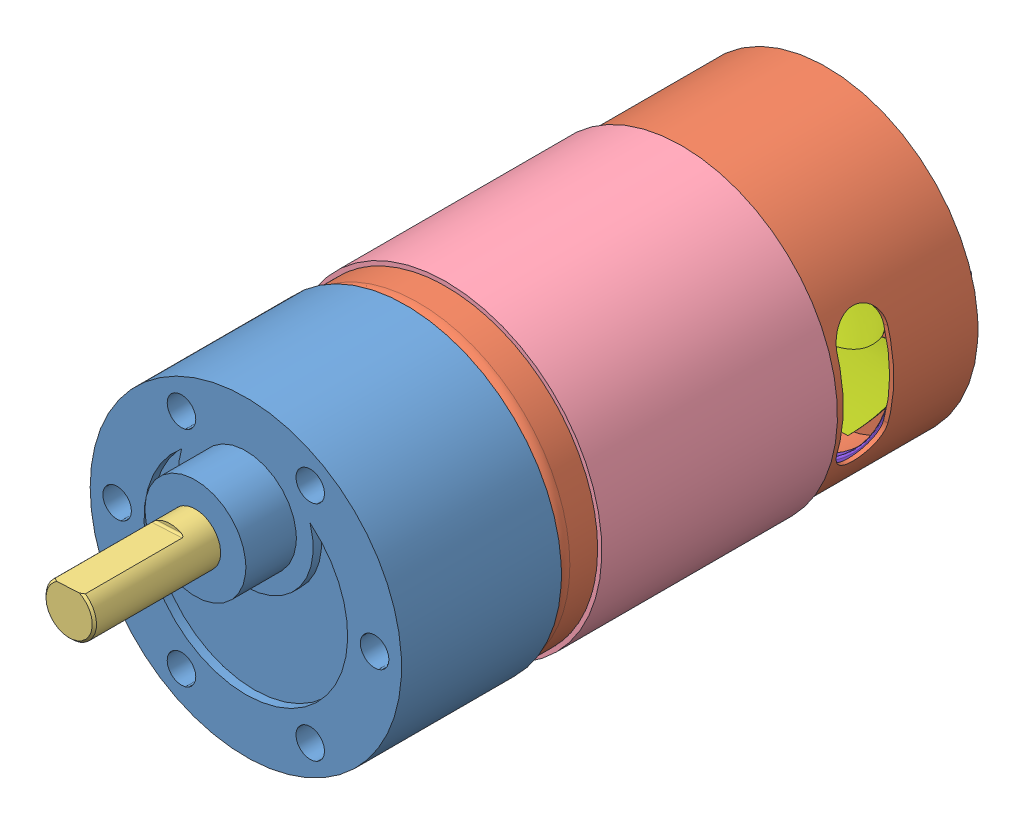
SolidWorks assembly Motor JGB37-545, configuration Predeterminado. Lengths in mm.
Overall size (37 37 94.88).
11 component instances, 11 part files, 33 mates.
Components (placement in the parent):
- Reduction box body-1: Reduction box body [Default] at (-12.375 1.5 54.875) size (37 37 25)
- Motor body-1: Motor body [Predeterminado] at (-12.375 1.5 4.875) size (36 36 52)
- Shaft-1: Shaft [Predeterminado] at (-12.375 8.5 67.775) x (0.998724 0.050497 0) z (0 0 1) size (6 6 27.1)
- Cover-1: Cover [Predeterminado] at (-12.375 1.5 22.075) size (37 36.74 28)
- Rotor-1: Rotor [Predeterminado] at (-12.375 1.5 32.275) x (0.999981 -0.006201 0) z (0 0 1) size (26 25.6 60)
- Magnets-1: Magnets [Default] at (-12.375 1.5 22.875) x (0 1 0) z (0 0 1) size (35 27.22 20)
- Fan-1: Fan [Default] at (-12.375 1.5 12.975) x (0.995635 -0.093332 0) z (0.093332 0.995635 0) size (31.79 6.24 31.22)
- Terminals-1: Terminals [Default] at (-12.375 1.5 5.375) x (1 0 0) z (0 0 -1) size (34 34 22.88)
- Gear 1-1: Gear 1 [Default] at (-12.375 1.5 62.275) x (-0.006201 -0.999981 0) z (0.999981 -0.006201 0) size (5.97 2 5.97)
- Gear 2-1: Gear 2 [Default] at (-12.375 -3.65 64.275) x (-0.919431 0.393252 0) z (-0.393252 -0.919431 0) size (20 8.6 20)
- Gear 3-1: Gear 3 [Default] at (-12.375 8.5 66.275) x (0.050497 -0.998724 0) z (0.998724 0.050497 0) size (10 10 9.98)
Mates (geometry in assembly coordinates):
- Coincidente1: coincident anti-aligned: plane of Reduction box body-1 through (-12.375 1.5 54.875) normal (0 0 -1); plane of Motor body-1 through (-12.375 1.5 54.875) normal (0 0 1)
- Concéntrica1: concentric aligned: cylinder of Reduction box body-1 through (-12.375 1.5 73.875) axis (0 0 -1) radius 18.5; cylinder of Motor body-1 through (-12.375 1.5 54.875) axis (0 0 -1) radius 18
- Distancia1: distance = 15 mm aligned: plane of Shaft-1 through (-12.375 8.5 94.875) normal (0 0 1); plane of GM37-3525_HT_Motor-1 through (-12.375 8.5 79.875) normal (0 0 1)
- Concéntrica2: concentric anti-aligned: cylinder of Reduction box body-1 through (-12.375 8.5 54.874) axis (0 0 1) radius 3; cylinder of Shaft-1 through (-12.375 8.5 94.875) axis (0 0 -1) radius 3
- Distancia2: distance = 4.8 mm anti-aligned: plane of Cover-1 through (-12.375 1.5 50.075) normal (0 0 1); plane of GM37-3525_HT_Motor-1 through (-12.375 1.5 54.875) normal (0 0 -1)
- Concéntrica3: concentric aligned: cylinder of Motor body-1 through (-12.375 1.5 54.875) axis (0 0 -1) radius 18; cylinder of Cover-1 through (-12.375 1.5 50.075) axis (0 0 -1) radius 18
- Concentric1: concentric aligned: cylinder of Motor body-1 through (-12.375 1.5 54.875) axis (0 0 -1) radius 17.5; cylinder of Rotor-1 through (-12.375 1.5 30.875) axis (0 0 -1) radius 13
- Distance1: distance = 4 mm aligned: plane of Rotor-1 through (-15.3249 1.5183 8.875) normal (0 0 -1); plane of Motor-1 through (-12.375 1.5 4.875) normal (0 0 -1)
- Concentric3: concentric aligned: cylinder of Motor body-1 through (-12.375 1.5 54.875) axis (0 0 -1) radius 17.5; cylinder of Magnets-1 through (-12.375 1.5 42.875) axis (0 0 -1) radius 14.5
- Distance4: distance = 2 mm aligned: plane of magnets-1 through (-12.375 1.5 22.875) normal (0 0 -1); plane of Rotor-1 through (-12.375 1.5 24.875) normal (0 0 -1)
- Parallel2: parallel aligned: plane of Magnets-1 through (1.2357 6.5 42.875) normal (1 0 0)
- Coincident9: coincident anti-aligned: plane of Rotor-1 through (-12.375 1.5 9.375) normal (0.999981 -0.006201 0); plane of Fan-1 through (-12.3567 4.4499 14.0996) normal (-0.999981 0.006201 0)
- Concentric5: concentric aligned: cylinder of Rotor-1 through (-12.375 1.5 62.275) axis (0 0 -1) radius 2; cylinder of Fan-1 through (-12.375 1.5 8.7004) axis (0 0 -1) radius 2
- Distance5: distance = 2 mm anti-aligned: plane of Rotor-1 through (-14.5478 4.2211 14.975) normal (0 0 -1); plane of Fan-1 through (-12.375 1.5 12.975) normal (0 0 1)
- Coincident13: coincident anti-aligned: plane of Motor body-1 through (-25.125 -0.5 15.375) normal (0 1 0); plane of Terminals-1 through (-25.125 -0.5 4.875) normal (0 -1 0)
- Coincident14: coincident anti-aligned: plane of Motor body-1 through (0.375 3.5 15.375) normal (-1 0 0); plane of Terminals-1 through (0.375 -0.5 4.875) normal (1 0 0)
- Coincident15: coincident aligned: plane of Motor body-1 through (-12.375 -16 5.875) normal (0 0 1); plane of Terminals-1 through (-12.375 1.5 5.875) normal (0 0 1)
- Coincident16: coincident anti-aligned: plane of Terminals-1 through (-25.125 0.9005 0) normal (0 0 -1)
- Coincident17: coincident aligned: plane of Terminals-1 through (0 3 6.875) normal (1 0 0)
- Coincident18: coincident anti-aligned: plane of Terminals-1 through (-0.75 0 6.875) normal (0 -1 0)
- Parallel3: parallel anti-aligned: plane of Cover-1 through (-9.275 -16.231 50.075) normal (-1 0 0)
- Parallel4: parallel aligned: plane of Reduction box body-1 through (-18.625 -12.75 55.025) normal (1 0 0)
- Concentric6: concentric anti-aligned: cylinder of Rotor-1 through (-12.375 1.5 62.275) axis (0 0 -1) radius 2; cylinder of Gear 1-1 through (-12.375 1.5 60.275) axis (0 0 1) radius 2
- Coincident19: coincident anti-aligned: plane of Rotor-1 through (-12.3657 3 56.275) normal (0.006201 0.999981 0); plane of Gear 1-1 through (-12.3657 3 60.275) normal (-0.006201 -0.999981 0)
- Coincident26: coincident aligned: plane of Rotor-1 through (-12.375 1.5 62.275) normal (0 0 1); plane of Gear 1-1 through (-12.375 1.5 62.275) normal (0 0 1)
- Concentric7: concentric anti-aligned: cylinder of Shaft-1 through (-12.375 8.5 94.875) axis (0 0 -1) radius 3; cylinder of Gear 5-1 through (-12.375 8.5 64.275) axis (0 0 1) radius 5
- Coincident23: coincident anti-aligned: plane of Shaft-1 through (-12.4129 9.249 70.275) normal (0.050497 -0.998724 0); plane of Gear 5-1 through (-12.4129 9.249 67.775) normal (-0.050497 0.998724 0)
- Coincident24: coincident anti-aligned: plane of Shaft-1 through (-12.375 8.5 70.275) normal (0 0 -1); plane of Gear 5-1 through (-12.375 8.5 70.275) normal (0 0 1)
- Parallel5: parallel anti-aligned: plane of Shaft-1 through (-12.375 8.5 94.875) normal (0 0 1); plane of Gear 2-1 through (-12.375 -3.65 58.275) normal (0 0 -1)
- Coincident27: coincident aligned: plane of Gear 1-1 through (-12.375 1.5 60.275) normal (0 0 -1); plane of Gear 2-1 through (-12.375 -3.65 60.275) normal (0 0 -1)
- Concentric9: concentric aligned: cylinder of Reduction box body-1 through (-12.375 -3.65 65.875) axis (0 0 1) radius 2; cylinder of Gear 2-1 through (-12.375 -3.65 58.275) axis (0 0 1) radius 1
- GearMate2: gear = 28 : 23 mm: cylinder of Gear 2-1 through (-12.375 -3.65 60.275) axis (0 0 1) radius 2.5; cylinder of Gear 1-1 through (-12.375 1.5 60.275) axis (0 0 1) radius 3
- GearMate3: gear = 23 : 100 mm: cylinder of Gear 2-1 through (-12.375 -3.65 64.275) axis (0 0 -1) radius 10; cylinder of Gear 3-1 through (-12.375 8.5 62.275) axis (0 0 1) radius 2.5
